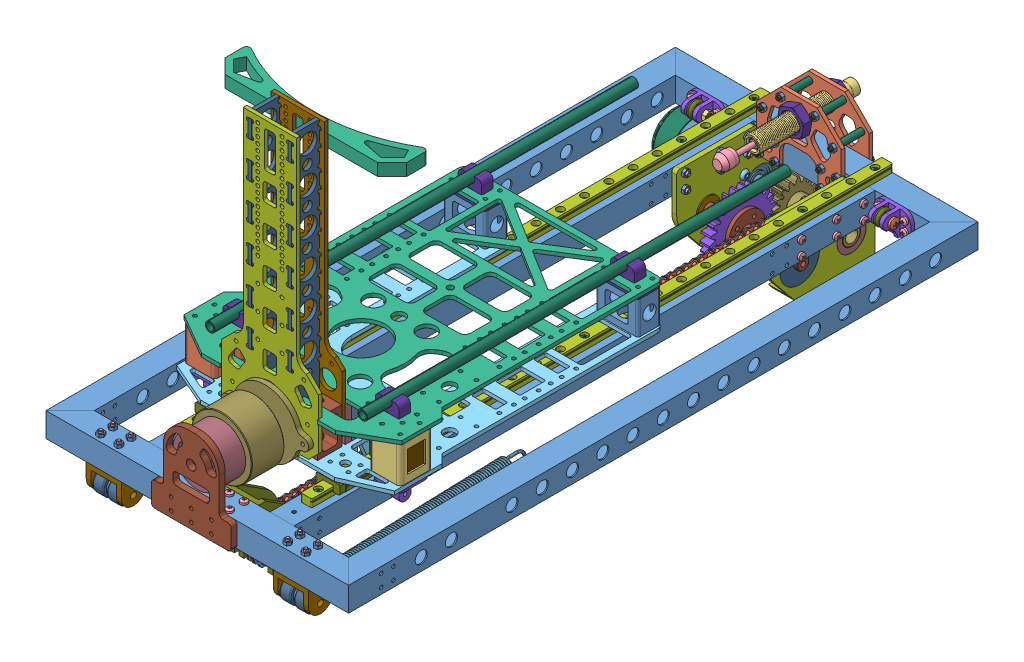
SolidWorks assembly 寒冰射手-wlⅡ-2AT-sc, configuration 默认. Lengths in mm. (continued)
Components (placement in the parent): (continued)
- 内链板T-sc-27: 内链板T-sc [默认] at (-33.1592 30.038 131.3321) x (0 0.000728 1) z (1 0 0) size (12.35 6 4.78)
- 内链板T-sc-28: 内链板T-sc [默认] at (-33.1592 30.0473 144.032) x (0 0.000728 1) z (1 0 0) size (12.35 6 4.78)
- 内链板T-sc-29: 内链板T-sc [默认] at (-33.1592 30.0565 156.732) x (0 0.000728 1) z (1 0 0) size (12.35 6 4.78)
- 内链板T-sc-30: 内链板T-sc [默认] at (-33.1592 30.0658 169.432) x (0 0.000728 1) z (1 0 0) size (12.35 6 4.78)
- 内链板T-sc-31: 内链板T-sc [默认] at (-33.1592 30.075 182.132) x (0 0.000728 1) z (1 0 0) size (12.35 6 4.78)
- 内链板T-sc-32: 内链板T-sc [默认] at (-33.1592 30.0843 194.832) x (0 0.000728 1) z (1 0 0) size (12.35 6 4.78)
- 内链板T-sc-33: 内链板T-sc [默认] at (-33.1592 30.0935 207.532) x (0 0.000728 1) z (1 0 0) size (12.35 6 4.78)
- 内链板T-sc-34: 内链板T-sc [默认] at (-33.1592 29.3036 220.1821) x (0 -0.470065 0.882632) z (1 0 0) size (12.35 6 4.78)
- 内链板T-sc-35: 内链板T-sc [默认] at (-33.1592 21.5108 229.9349) x (0 -0.941992 0.335634) z (1 0 0) size (12.35 6 4.78)
- 内链板T-sc-36: 内链板T-sc [默认] at (-33.1592 9.1815 231.8928) x (0 -0.922274 -0.386537) z (1 0 0) size (12.35 6 4.78)
- 内链板T-sc-37: 内链板T-sc [默认] at (-33.1592 -1.2493 225.0341) x (0 -0.421201 -0.906967) z (1 0 0) size (12.35 6 4.78)
- 内链板T-sc-38: 内链板T-sc [默认] at (-33.1592 -4.4596 212.9475) x (0 0.000726 -1) z (1 0 0) size (12.35 6 4.78)
- 内链板T-sc-39: 内链板T-sc [默认] at (-33.1592 -4.4503 200.2475) x (0 0.000726 -1) z (1 0 0) size (12.35 6 4.78)
- 内链板T-sc-40: 内链板T-sc [默认] at (-33.1592 -4.4411 187.5475) x (0 0.000726 -1) z (1 0 0) size (12.35 6 4.78)
- 内链板T-sc-41: 内链板T-sc [默认] at (-33.1592 -4.4319 174.8475) x (0 0.000726 -1) z (1 0 0) size (12.35 6 4.78)
- 内链板T-sc-42: 内链板T-sc [默认] at (-33.1592 -4.4227 162.1475) x (0 0.000726 -1) z (1 0 0) size (12.35 6 4.78)
- 内链板T-sc-43: 内链板T-sc [默认] at (-33.1592 -4.4135 149.4475) x (0 0.000726 -1) z (1 0 0) size (12.35 6 4.78)
- 内链板T-sc-44: 内链板T-sc [默认] at (-33.1592 -4.4042 136.7475) x (0 0.000726 -1) z (1 0 0) size (12.35 6 4.78)
- 内链板T-sc-45: 内链板T-sc [默认] at (-33.1592 -4.395 124.0475) x (0 0.000726 -1) z (1 0 0) size (12.35 6 4.78)
- 内链板T-sc-46: 内链板T-sc [默认] at (-33.1592 -4.3858 111.3475) x (0 0.000726 -1) z (1 0 0) size (12.35 6 4.78)
- 内链板T-sc-47: 内链板T-sc [默认] at (-33.1592 -4.3766 98.6476) x (0 0.000726 -1) z (1 0 0) size (12.35 6 4.78)
- 内链板T-sc-48: 内链板T-sc [默认] at (-33.1592 -4.3674 85.9476) x (0 0.000726 -1) z (1 0 0) size (12.35 6 4.78)
- 内链板T-sc-49: 内链板T-sc [默认] at (-33.1592 -4.3581 73.2476) x (0 0.000726 -1) z (1 0 0) size (12.35 6 4.78)
- 内链板T-sc-50: 内链板T-sc [默认] at (-33.1592 -4.3489 60.5476) x (0 0.000726 -1) z (1 0 0) size (12.35 6 4.78)
- 内链板T-sc-51: 内链板T-sc [默认] at (-33.1592 -4.3397 47.8476) x (0 0.000726 -1) z (1 0 0) size (12.35 6 4.78)
- 内链板T-sc-52: 内链板T-sc [默认] at (-33.1592 -4.3305 35.1476) x (0 0.000726 -1) z (1 0 0) size (12.35 6 4.78)
- 内链板T-sc-53: 内链板T-sc [默认] at (-33.1592 -4.3212 22.4476) x (0 0.000726 -1) z (1 0 0) size (12.35 6 4.78)
- 内链板T-sc-54: 内链板T-sc [默认] at (-33.1592 -4.312 9.7476) x (0 0.000726 -1) z (1 0 0) size (12.35 6 4.78)
- 内链板T-sc-55: 内链板T-sc [默认] at (-33.1592 -4.3028 -2.9524) x (0 0.000726 -1) z (1 0 0) size (12.35 6 4.78)
- 内链板T-sc-56: 内链板T-sc [默认] at (-33.1592 -4.2936 -15.6524) x (0 0.000726 -1) z (1 0 0) size (12.35 6 4.78)
- 内链板T-sc-57: 内链板T-sc [默认] at (-33.1592 -4.2844 -28.3523) x (0 0.000726 -1) z (1 0 0) size (12.35 6 4.78)
- 内链板T-sc-58: 内链板T-sc [默认] at (-33.1592 -4.2751 -41.0523) x (0 0.000726 -1) z (1 0 0) size (12.35 6 4.78)
- 内链板T-sc-59: 内链板T-sc [默认] at (-33.1592 -4.2659 -53.7523) x (0 0.000726 -1) z (1 0 0) size (12.35 6 4.78)
- 内链板T-sc-60: 内链板T-sc [默认] at (-33.1592 -4.2567 -66.4523) x (0 0.000726 -1) z (1 0 0) size (12.35 6 4.78)
- 内链板T-sc-61: 内链板T-sc [默认] at (-33.1592 -4.2475 -79.1523) x (0 0.000726 -1) z (1 0 0) size (12.35 6 4.78)
- 内链板T-sc-62: 内链板T-sc [默认] at (-33.1592 -4.2383 -91.8523) x (0 0.000726 -1) z (1 0 0) size (12.35 6 4.78)
- 内链板T-sc-63: 内链板T-sc [默认] at (-33.1592 -4.229 -104.5523) x (0 0.000726 -1) z (1 0 0) size (12.35 6 4.78)
- 内链板T-sc-64: 内链板T-sc [默认] at (-33.1592 -4.2198 -117.2523) x (0 0.000726 -1) z (1 0 0) size (12.35 6 4.78)
- 内链板T-sc-65: 内链板T-sc [默认] at (-33.1592 -4.2106 -129.9523) x (0 0.000726 -1) z (1 0 0) size (12.35 6 4.78)
- 内链板T-sc-66: 内链板T-sc [默认] at (-33.1592 -4.2014 -142.6522) x (0 0.000726 -1) z (1 0 0) size (12.35 6 4.78)
- 内链板T-sc-67: 内链板T-sc [默认] at (-33.1592 -4.1922 -155.3522) x (0 0.000726 -1) z (1 0 0) size (12.35 6 4.78)
- 内链板T-sc-68: 内链板T-sc [默认] at (-33.1592 -4.1829 -168.0522) x (0 0.000726 -1) z (1 0 0) size (12.35 6 4.78)
- 内链板T-sc-69: 内链板T-sc [默认] at (-33.1592 -4.1737 -180.7522) x (0 0.000726 -1) z (1 0 0) size (12.35 6 4.78)
- 内链板T-sc-70: 内链板T-sc [默认] at (-33.1592 -4.1645 -193.4522) x (0 0.02154 -0.999768) z (1 0 0) size (12.35 6 4.78)
- 内链板T-sc-71: 内链板T-sc [默认] at (-33.1592 -2.0684 -205.8409) x (0 0.636425 -0.771338) z (1 0 0) size (12.35 6 4.78)
- 内链板T-sc-72: 内链板T-sc [默认] at (-33.1592 7.531 -213.8097) x (0 0.991746 -0.12822) z (1 0 0) size (12.35 6 4.78)
- 内链板T-sc-73: 内链板T-sc [默认] at (-33.1592 19.9849 -213.0676) x (0 0.811669 0.584118) z (1 0 0) size (12.35 6 4.78)
- 链齿平钩T-1: 链齿平钩T [默认] at (-33.1492 30.127 90.8901) x (0 -0.000728 -1) z (-1 0 0) size (27.4 8.17 29)
- 链齿平钩下-1: 链齿平钩下 [默认] at (-33.1492 29.8726 66.771) x (0 0.000728 1) z (-1 0 0) size (27.4 4 29)
- 发射托盘-wlⅡ-1: 发射托盘-wlⅡ [默认] at (-17.4385 -21.9121 -45.4891) size (180 275 367.06)
  - 发射托盘-wlⅡ11-1: 发射托盘-wlⅡ11 [默认] at (25.4712 86.7307 214.002) x (1 0 0) z (0 1 0) size (180 367.06 246)
    - 发射下平台-wlⅡ11-1: 发射下平台-wlⅡ11 [默认] at (129.5435 38.08 -1.5) size (180 244.52 3)
    - 发射上平台-wlⅡ11-1: 发射上平台-wlⅡ11 [默认] at (-66.2821 39.0561 31.5) x (-1 0 0) z (0 0 1) size (180 243.55 3)
    - 后推板-wlⅡ11-1: 后推板-wlⅡ11 [默认] at (-54.3543 -31.5036 108.5) x (-1 0 0) z (0 0 -1) size (80 3 230)
    - 弹射拉线小座子-wlⅡ11-1: 弹射拉线小座子-wlⅡ11 [默认] at (-136.5321 -0.5634 -1.5) x (0 -1 0) z (1 0 0) size (24 18 23)
    - 弹射拉线小座子-wlⅡ11-2: 弹射拉线小座子-wlⅡ11 [默认] at (17.9679 -0.5634 -1.5) x (0 -1 0) z (1 0 0) size (24 18 23)
    - 前推板-wlⅡ11-1: 前推板-wlⅡ11 [默认] at (-19.2821 -8.5036 1.5) x (-1 0 0) z (0 0 -1) size (73 3 218)
    - 侧向加固板-wlⅡ11-1: 侧向加固板-wlⅡ11 [默认] at (-41.2821 -8.5036 31.6) x (0 -1 0) z (0 0 -1) size (26 3 194.4)
    - 侧向加固板-wlⅡ11-2: 侧向加固板-wlⅡ11 [默认] at (-74.2821 -8.5036 31.6) x (0 -1 0) z (0 0 -1) size (26 3 194.4)
    - 推板固定件-wlⅡ11-1: 推板固定件-wlⅡ11 [默认] at (-22.7821 -18.5036 16.5) x (0 -1 0) z (-1 0 0) size (20 30 73)
    - 电磁吸铁80kg配套-wlⅡ11-1: 电磁吸铁80kg配套-wlⅡ11 [默认] at (-59.2821 -35.5036 14) x (1 0 0) z (0 1 0) size (72 54 4)
    - 8mm发泡硅胶-wlⅡ11-1: 8mm发泡硅胶-wlⅡ11 [默认] at (-59.2821 -8.5036 16.5) size (73 8 30)
    - 8mm聚氨酯-wlⅡ11-1: 8mm聚氨酯-wlⅡ11 [默认] at (-59.2821 -0.5036 16.5) size (73 8 30)
    - 碳管300-wlⅡ11-1: 碳管300-wlⅡ11 [默认] at (-121.7821 331.5561 42.5) x (1 0 0) z (0 -1 0) size (8 8 350)
    - 碳管300-wlⅡ11-2: 碳管300-wlⅡ11 [默认] at (4.2179 331.5561 42.5) x (0.546685 0 0.837338) z (0 -1 0) size (8 8 350)
    - 纵向滑块9mm-wlⅡ11-1: 纵向滑块9mm-wlⅡ11 [默认] at (-109.2822 -33.5634 -9.5) x (1 0 0) z (0 -1 0) size (20 8 28.9)
    - 纵向滑块9mm-wlⅡ11-2: 纵向滑块9mm-wlⅡ11 [默认] at (-9.2819 -33.5634 -9.5) x (1 0 0) z (0 -1 0) size (20 8 28.9)
    - 纵向滑块9mm-wlⅡ11-3: 纵向滑块9mm-wlⅡ11 [默认] at (-109.2822 32.5366 -9.5) x (1 0 0) z (0 -1 0) size (20 8 28.9)
    - 纵向滑块9mm-wlⅡ11-4: 纵向滑块9mm-wlⅡ11 [默认] at (-9.2819 32.5366 -9.5) x (1 0 0) z (0 -1 0) size (20 8 28.9)
    - 碳管夹2改1-1: 碳管夹2改1 [默认] at (4.2179 6.5561 28.5) x (0 1 0) z (0 0 1) size (19 35 16)
    - 垫块1-1: 垫块1 [默认] at (17.9679 -0.5634 1.5) x (0 -1 0) z (0 0 1) size (23 22 30)
    - 碳管夹2改1-2: 碳管夹2改1 [默认] at (4.2179 201.0156 28.5) x (0 1 0) z (0 0 1) size (19 35 16)
    - 垫块改1-1: 垫块改1 [默认] at (4.2179 201.0156 1.5) size (35 19 27)
    - 方碳管固定1-1: 方碳管固定1 [默认] at (-130.2821 1.5561 1.5) size (37 30 30)
    - 方碳管固定右1-2: 方碳管固定右1 [默认] at (11.7179 1.5561 31.5) x (-1 0 0) z (0 0 -1) size (37 30 30)
    - 加固碳板1-1: 加固碳板1 [默认] at (-42.2822 22.9964 -4.5) size (35 50 3)
  - 平台直钩1-1: 平台直钩1 [默认] at (-16.811 82.2307 191.0056) x (1 0 0) z (0 -1 0) size (26 20 44)
  - 垫块改1-1: 垫块改1 [默认] at (-96.3109 88.2307 12.9864) x (1 0 0) z (0 1 0) size (35 19 27)
  - 碳管夹2改1-1: 碳管夹2改1 [默认] at (-96.3109 115.2307 12.9864) x (0 0 -1) z (0 1 0) size (19 35 16)
  - 碳管夹2改1-2: 碳管夹2改1 [默认] at (-96.3109 115.2307 207.4459) x (0 0 -1) z (0 1 0) size (19 35 16)
  - 小推爪-280--1: 小推爪-280- [默认] at (-33.8109 293.2307 204.9956) size (150 10 29.67)
Mates (geometry in assembly coordinates):
- 重合1: coincident anti-aligned: plane of 发射架-wlⅡ-2AT-sc-1 through (63.7508 32.8186 -260) normal (0 0 -1); plane of 缓冲器固定板-wlⅡ-2AT-sc-1 through (-86.2492 32.8186 -260) normal (0 0 1)
- 重合2: coincident aligned: plane of 发射架-wlⅡ-2AT-sc-1 through (63.7508 32.8186 -240) normal (0 -1 0); plane of 缓冲器固定板-wlⅡ-2AT-sc-1 through (-86.2492 32.8186 -260) normal (0 -1 0)
- 宽度1: width anti-aligned: plane of 发射架-wlⅡ-2AT-sc-1 through (-91.2492 32.8186 250) normal (1 0 0); plane of 发射架-wlⅡ-2AT-sc-1 through (-11.2492 32.8186 250) normal (-1 0 0); plane of 缓冲器固定板-wlⅡ-2AT-sc-1 through (-86.2492 32.8186 -260) normal (-1 0 0); plane of 缓冲器固定板-wlⅡ-2AT-sc-1 through (-16.2492 32.8186 -260) normal (1 0 0)
- 重合4: coincident anti-aligned: plane of 发射架-wlⅡ-2AT-sc-1 through (63.7508 32.8186 -240) normal (0 0 1); plane of 缓冲器固定板-wlⅡ-2AT-sc-3 through (-86.2492 32.8186 -240) normal (0 0 -1)
- 重合5: coincident aligned: plane of 发射架-wlⅡ-2AT-sc-1 through (63.7508 32.8186 -240) normal (0 -1 0); plane of 缓冲器固定板-wlⅡ-2AT-sc-3 through (-86.2492 32.8186 -237) normal (0 -1 0)
- 重合6: coincident aligned: plane of 缓冲器固定板-wlⅡ-2AT-sc-1 through (-16.2492 32.8186 -260) normal (1 0 0); plane of 缓冲器固定板-wlⅡ-2AT-sc-3 through (-16.2492 32.8186 -237) normal (1 0 0)
- 同心1: concentric aligned: cylinder of 缓冲器固定板-wlⅡ-2AT-sc-3 through (-51.2492 76.3186 -237) axis (0 0 -1) radius 7; cylinder of 阻尼器-wlⅡ-2AT-sc-1/阻尼器缸体-wlⅡ-2AT-sc-1 through (-51.2492 76.3186 -270) axis (0 0 -1) radius 5.875
- 同心2: concentric aligned: cylinder of 缓冲器固定板-wlⅡ-2AT-sc-1 through (-51.2492 76.3186 -260) axis (0 0 -1) radius 7; cylinder of GB／T6172．1-2000六角薄螺母A级和B级(M14)-wlⅡ-2AT-sc-1 through (-51.2492 76.3186 -263) axis (0 0 -1) radius 7
- 重合7: coincident anti-aligned: plane of 缓冲器固定板-wlⅡ-2AT-sc-1 through (-86.2492 32.8186 -263) normal (0 0 -1); plane of GB／T6172．1-2000六角薄螺母A级和B级(M14)-wlⅡ-2AT-sc-1 through (-49.1953 87.8115 -263) normal (0 0 1)
- 重合9: coincident aligned: circle of 阻尼器-wlⅡ-2AT-sc-1/阻尼器缸体-wlⅡ-2AT-sc-1; plane of GB／T6172．1-2000六角薄螺母A级和B级(M14)-wlⅡ-2AT-sc-1 through (-49.1953 87.8115 -270) normal (0 0 -1)
- 同心4: concentric aligned: cylinder of 阻尼器-wlⅡ-2AT-sc-1/阻尼器缸体-wlⅡ-2AT-sc-1 through (-51.2492 76.3186 -276.1) axis (0 0 -1) radius 5.875; cylinder of GB／T6172．1-2000六角薄螺母A级和B级(M14)-wlⅡ-2AT-sc-2 through (-51.2492 76.3186 -230) axis (0 0 -1) radius 7
- 重合10: coincident anti-aligned: plane of 缓冲器固定板-wlⅡ-2AT-sc-3 through (-86.2492 32.8186 -237) normal (0 0 1); plane of GB／T6172．1-2000六角薄螺母A级和B级(M14)-wlⅡ-2AT-sc-2 through (-49.1953 87.8115 -237) normal (0 0 -1)
- 重合11: coincident anti-aligned: plane of 发射架-wlⅡ-2AT-sc-1 through (-11.2492 52.8186 250) normal (0 1 0); plane of 发射导轨-wlⅡ-2AT-sc-1 through (-5.7492 52.8186 220) normal (0 -1 0)
- 重合14: coincident anti-aligned: plane of 发射架-wlⅡ-2AT-sc-1 through (-111.2492 52.8186 250) normal (0 1 0); plane of 发射导轨-wlⅡ-2AT-sc-2 through (-105.7492 52.8186 220) normal (0 -1 0)
- 宽度2: width anti-aligned: plane of 发射导轨-wlⅡ-2AT-sc-2 through (-105.7492 52.8186 220) normal (-1 0 0); plane of 发射导轨-wlⅡ-2AT-sc-2 through (-96.7492 52.8186 220) normal (1 0 0); plane of 发射架-wlⅡ-2AT-sc-1 through (-91.2492 32.8186 250) normal (1 0 0); plane of 发射架-wlⅡ-2AT-sc-1 through (-111.2492 32.8186 250) normal (-1 0 0)
- 宽度3: width anti-aligned: plane of 发射架-wlⅡ-2AT-sc-1 through (-11.2492 32.8186 250) normal (-1 0 0); plane of 发射架-wlⅡ-2AT-sc-1 through (8.7508 32.8186 250) normal (1 0 0); plane of 发射导轨-wlⅡ-2AT-sc-1 through (3.2508 52.8186 220) normal (1 0 0); plane of 发射导轨-wlⅡ-2AT-sc-1 through (-5.7492 52.8186 220) normal (-1 0 0)
- 重合15: coincident anti-aligned: plane of 缓冲器固定板-wlⅡ-2AT-sc-1 through (-86.2492 32.8186 -260) normal (0 0 1); plane of 20尼龙柱-wlⅡ-2AT-sc-1 through (-65.1781 84.8186 -260) normal (0 0 -1)
- 同心5: concentric anti-aligned: cylinder of 缓冲器固定板-wlⅡ-2AT-sc-1 through (-65.1781 84.8186 -260) axis (0 0 -1) radius 1.5; cylinder of 20尼龙柱-wlⅡ-2AT-sc-1 through (-65.1781 84.8186 -260) axis (0 0 1) radius 1.5
- 同心6: concentric anti-aligned: cylinder of 缓冲器固定板-wlⅡ-2AT-sc-1 through (-80.2492 69.7475 -260) axis (0 0 -1) radius 1.5; cylinder of 20尼龙柱-wlⅡ-2AT-sc-3 through (-80.2492 69.7475 -260) axis (0 0 1) radius 1.5
- 重合16: coincident anti-aligned: plane of 缓冲器固定板-wlⅡ-2AT-sc-1 through (-86.2492 32.8186 -260) normal (0 0 1); plane of 20尼龙柱-wlⅡ-2AT-sc-3 through (-80.2492 69.7475 -260) normal (0 0 -1)
- 同心7: concentric anti-aligned: cylinder of 缓冲器固定板-wlⅡ-2AT-sc-3 through (-37.3203 84.8186 -237) axis (0 0 -1) radius 1.5; cylinder of 20尼龙柱-wlⅡ-2AT-sc-4 through (-37.3203 84.8186 -260) axis (0 0 1) radius 1.5
- 重合17: coincident anti-aligned: plane of 缓冲器固定板-wlⅡ-2AT-sc-1 through (-86.2492 32.8186 -260) normal (0 0 1); plane of 20尼龙柱-wlⅡ-2AT-sc-4 through (-37.3203 84.8186 -260) normal (0 0 -1)
- 同心8: concentric anti-aligned: cylinder of 缓冲器固定板-wlⅡ-2AT-sc-1 through (-22.2492 69.7475 -260) axis (0 0 -1) radius 1.5; cylinder of 20尼龙柱-wlⅡ-2AT-sc-2 through (-22.2492 69.7475 -260) axis (0 0 1) radius 1.5
- 重合18: coincident anti-aligned: plane of 缓冲器固定板-wlⅡ-2AT-sc-1 through (-86.2492 32.8186 -260) normal (0 0 1); plane of 20尼龙柱-wlⅡ-2AT-sc-2 through (-22.2492 69.7475 -260) normal (0 0 -1)
- 重合19: coincident anti-aligned: plane of 发射架-wlⅡ-2AT-sc-1 through (63.7508 32.8186 -240) normal (0 0 1); plane of 拉线座子-wlⅡ-2AT-sc-1 through (26.0008 52.8186 -240) normal (0 0 -1)
- 重合20: coincident aligned: plane of 发射架-wlⅡ-2AT-sc-1 through (63.7508 32.8186 -240) normal (0 -1 0); plane of 拉线座子-wlⅡ-2AT-sc-1 through (45.3335 32.8186 -223) normal (0 -1 0)
- 重合21: coincident anti-aligned: plane of 发射架-wlⅡ-2AT-sc-1 through (63.7508 32.8186 -240) normal (0 0 1); plane of 拉线座子-wlⅡ-2AT-sc-2 through (-128.4992 52.8186 -240) normal (0 0 -1)
- 重合22: coincident aligned: plane of 发射架-wlⅡ-2AT-sc-1 through (63.7508 52.8186 -240) normal (0 1 0); plane of 拉线座子-wlⅡ-2AT-sc-2 through (-128.4992 52.8186 -231.5) normal (0 1 0)
- 距离1: distance = 2 mm anti-aligned: plane of 发射架-wlⅡ-2AT-sc-1 through (-111.2492 32.8186 250) normal (-1 0 0); plane of 拉线座子-wlⅡ-2AT-sc-2 through (-113.2492 25.8186 -237) normal (1 0 0)
- 距离2: distance = 2 mm anti-aligned: plane of 发射架-wlⅡ-2AT-sc-1 through (8.7508 32.8186 250) normal (1 0 0); plane of 拉线座子-wlⅡ-2AT-sc-1 through (10.7508 25.8186 -237) normal (-1 0 0)
- 同心9: concentric aligned: cylinder of 拉线座子-wlⅡ-2AT-sc-2 through (-122.2492 46.0686 -231) axis (-1 0 0) radius 2; cylinder of 现有线轮轴承-wlⅡ-2AT-sc-1 through (-194.9309 46.0686 -231) axis (-1 0 0) radius 2
- 同心10: concentric aligned: cylinder of 拉线座子-wlⅡ-2AT-sc-1 through (32.2508 46.0686 -231) axis (-1 0 0) radius 2; cylinder of 现有线轮轴承-wlⅡ-2AT-sc-2 through (-40.4309 46.0686 -231) axis (-1 0 0) radius 2
- 宽度4: width anti-aligned: plane of 拉线座子-wlⅡ-2AT-sc-2 through (-131.7492 52.8186 -231.5) normal (1 0 0); plane of 拉线座子-wlⅡ-2AT-sc-2 through (-125.2492 52.8186 -231.5) normal (-1 0 0); plane of 现有线轮轴承-wlⅡ-2AT-sc-1 through (-131.4992 48.0684 -231.0238) normal (-1 0 0); plane of 现有线轮轴承-wlⅡ-2AT-sc-1 through (-125.4992 48.0684 -231.0238) normal (1 0 0)
- 宽度6: width anti-aligned: plane of 拉线座子-wlⅡ-2AT-sc-1 through (29.2508 52.8186 -231.5) normal (-1 0 0); plane of 拉线座子-wlⅡ-2AT-sc-1 through (22.7508 52.8186 -231.5) normal (1 0 0); plane of 现有线轮轴承-wlⅡ-2AT-sc-2 through (29.0008 48.0574 -230.7888) normal (1 0 0); plane of 现有线轮轴承-wlⅡ-2AT-sc-2 through (23.0008 48.0574 -230.7888) normal (-1 0 0)
- 宽度7: width anti-aligned: plane of 拉簧座子-wlⅡ-2AT-sc-1 through (36.5008 10.8186 260) normal (-1 0 0); plane of 拉簧座子-wlⅡ-2AT-sc-1 through (15.5008 10.8186 240) normal (1 0 0); plane of 拉线座子-wlⅡ-2AT-sc-1 through (19.7508 52.8186 -231.5) normal (-1 0 0); plane of 拉线座子-wlⅡ-2AT-sc-1 through (32.2508 52.8186 -231.5) normal (1 0 0)
- 宽度8: width anti-aligned: plane of 拉簧座子-wlⅡ-2AT-sc-2 through (-117.9992 10.8186 260) normal (-1 0 0); plane of 拉簧座子-wlⅡ-2AT-sc-2 through (-138.9992 10.8186 240) normal (1 0 0); plane of 拉线座子-wlⅡ-2AT-sc-2 through (-134.7492 52.8186 -231.5) normal (-1 0 0); plane of 拉线座子-wlⅡ-2AT-sc-2 through (-122.2492 52.8186 -231.5) normal (1 0 0)
- 重合27: coincident anti-aligned: plane of 拉簧座子-wlⅡ-2AT-sc-2 through (-138.9992 10.8186 240) normal (1 0 0); plane of 弹簧限位件-wlⅡ-2AT-sc-1 through (-138.9992 18.3186 250) normal (-1 0 0)
- 同心11: concentric anti-aligned: cylinder of 拉簧座子-wlⅡ-2AT-sc-2 through (-113.9992 18.3186 250) axis (-1 0 0) radius 2.5; cylinder of 弹簧限位件-wlⅡ-2AT-sc-1 through (-138.9992 18.3186 250) axis (1 0 0) radius 4.15
- 同心12: concentric anti-aligned: cylinder of 拉簧座子-wlⅡ-2AT-sc-2 through (-113.9992 18.3186 250) axis (-1 0 0) radius 2.5; cylinder of 弹簧限位件-wlⅡ-2AT-sc-2 through (-126.9992 18.3186 250) axis (1 0 0) radius 4.15
- 重合28: coincident anti-aligned: plane of 拉簧座子-wlⅡ-2AT-sc-2 through (-117.9992 10.8186 260) normal (-1 0 0); plane of 弹簧限位件-wlⅡ-2AT-sc-2 through (-117.9992 18.3186 250) normal (1 0 0)
- 同心13: concentric anti-aligned: cylinder of 拉簧座子-wlⅡ-2AT-sc-1 through (40.5008 18.3186 250) axis (-1 0 0) radius 2.5; cylinder of 弹簧限位件-wlⅡ-2AT-sc-3 through (27.5008 18.3186 250) axis (1 0 0) radius 4.15
- 重合29: coincident anti-aligned: plane of 拉簧座子-wlⅡ-2AT-sc-1 through (36.5008 10.8186 260) normal (-1 0 0); plane of 弹簧限位件-wlⅡ-2AT-sc-3 through (36.5008 18.3186 250) normal (1 0 0)
- 重合30: coincident anti-aligned: plane of 拉簧座子-wlⅡ-2AT-sc-1 through (15.5008 10.8186 240) normal (1 0 0); plane of 弹簧限位件-wlⅡ-2AT-sc-4 through (15.5008 18.3186 250) normal (-1 0 0)
- 同心14: concentric anti-aligned: cylinder of 拉簧座子-wlⅡ-2AT-sc-1 through (40.5008 18.3186 250) axis (-1 0 0) radius 2.5; cylinder of 弹簧限位件-wlⅡ-2AT-sc-4 through (15.5008 18.3186 250) axis (1 0 0) radius 4.15
- 重合31: coincident aligned: plane of 发射架-wlⅡ-2AT-sc-1 through (63.7508 32.8186 -260) normal (0 0 -1); plane of 发射导轨-wlⅡ-2AT-sc-2 through (-101.2492 56.482 -260) normal (0 0 -1)
- 重合32: coincident aligned: plane of 发射架-wlⅡ-2AT-sc-1 through (63.7508 32.8186 -260) normal (0 0 -1); plane of 发射导轨-wlⅡ-2AT-sc-1 through (-1.2492 56.482 -260) normal (0 0 -1)
- 重合33: coincident anti-aligned: plane of 电磁吸盘固定板-wlⅡ-2AT-sc-1 through (-51.2492 67.8186 260) normal (0 0 -1); plane of 发射架-wlⅡ-2AT-sc-1 through (-166.2492 32.8186 260) normal (0 0 1)
- 宽度9: width aligned: plane of 发射架-wlⅡ-2AT-sc-1 through (-11.2492 32.8186 250) normal (-1 0 0); plane of 发射架-wlⅡ-2AT-sc-1 through (-91.2492 32.8186 250) normal (1 0 0); plane of 电磁吸盘固定板-wlⅡ-2AT-sc-1 through (-74.2492 102.8186 260) normal (-1 0 0); plane of 电磁吸盘固定板-wlⅡ-2AT-sc-1 through (-28.2492 102.8186 260) normal (1 0 0)
- 同心15: concentric aligned: cylinder of 电磁吸盘固定板-wlⅡ-2AT-sc-1 through (-51.2492 78.8186 260) axis (0 0 1) radius 4; cylinder of 电磁铁开关80kg-wlⅡ-2AT-sc-1 through (-51.2492 78.8186 228) axis (0 0 1) radius 4
- 重合40: coincident aligned: plane of 发射架-wlⅡ-2AT-sc-1 through (-166.2492 32.8186 240) normal (0 -1 0); plane of 电磁吸盘固定板-wlⅡ-2AT-sc-1 through (-74.2492 32.8186 260) normal (0 -1 0)
- 重合41: coincident anti-aligned: plane of 发射架-wlⅡ-2AT-sc-1 through (-166.2492 32.8186 240) normal (0 -1 0); plane of 拉簧座子-wlⅡ-2AT-sc-1 through (26.0008 32.8186 250) normal (0 1 0)
- 重合42: coincident aligned: plane of 发射架-wlⅡ-2AT-sc-1 through (-166.2492 32.8186 260) normal (0 0 1); plane of 拉簧座子-wlⅡ-2AT-sc-1 through (26.0008 28.8186 260) normal (0 0 1)
- 重合43: coincident anti-aligned: plane of 发射架-wlⅡ-2AT-sc-1 through (-166.2492 32.8186 240) normal (0 -1 0); plane of 拉簧座子-wlⅡ-2AT-sc-2 through (-128.4992 32.8186 250) normal (0 1 0)
- 重合44: coincident aligned: plane of 发射架-wlⅡ-2AT-sc-1 through (-166.2492 32.8186 260) normal (0 0 1); plane of 拉簧座子-wlⅡ-2AT-sc-2 through (-128.4992 28.8186 260) normal (0 0 1)
- 同心17: concentric anti-aligned: cylinder of 电磁吸盘固定板-wlⅡ-2AT-sc-1 through (-51.2492 78.8186 260) axis (0 0 1) radius 4; cylinder of 行程调节块-wlⅡ-2AT-sc-1 through (-51.2492 78.8186 260) axis (0 0 -1) radius 4
- 重合49: coincident anti-aligned: plane of 电磁吸盘固定板-wlⅡ-2AT-sc-1 through (-51.2492 67.8186 260) normal (0 0 -1); plane of 行程调节块-wlⅡ-2AT-sc-1 through (-51.2492 78.8186 260) normal (0 0 1)
- 重合50: coincident anti-aligned: plane of 电磁铁开关80kg-wlⅡ-2AT-sc-1 through (-51.2492 78.8186 240) normal (0 0 1); plane of 行程调节块-wlⅡ-2AT-sc-1 through (-51.2492 78.8186 240) normal (0 0 -1)
- 同心26: concentric aligned: cylinder of 缓冲器固定板-wlⅡ-2AT-sc-1 through (-65.1781 84.8186 -260) axis (0 0 -1) radius 1.5; cylinder of GB／T818-2000十字槽盘头螺钉M3×30-wlⅡ-2AT-sc-1 through (-65.1781 84.8186 -266.7318) axis (0 0 -1) radius 1.5
- 重合71: coincident anti-aligned: plane of 缓冲器固定板-wlⅡ-2AT-sc-1 through (-86.2492 32.8186 -263) normal (0 0 -1); plane of GB／T818-2000十字槽盘头螺钉M3×30-wlⅡ-2AT-sc-1 through (-66.6512 85.853 -263) normal (0 0 1)
- 同心27: concentric aligned: cylinder of 缓冲器固定板-wlⅡ-2AT-sc-1 through (-80.2492 69.7475 -260) axis (0 0 -1) radius 1.5; cylinder of GB／T818-2000十字槽盘头螺钉M3×30-wlⅡ-2AT-sc-2 through (-80.2492 69.7475 -266.7318) axis (0 0 -1) radius 1.5
- 同心28: concentric aligned: cylinder of 缓冲器固定板-wlⅡ-2AT-sc-1 through (-37.3203 84.8186 -260) axis (0 0 -1) radius 1.5; cylinder of GB／T818-2000十字槽盘头螺钉M3×30-wlⅡ-2AT-sc-3 through (-37.3203 84.8186 -266.7318) axis (0 0 -1) radius 1.5
- 同心29: concentric aligned: cylinder of 缓冲器固定板-wlⅡ-2AT-sc-1 through (-22.2492 69.7475 -260) axis (0 0 -1) radius 1.5; cylinder of GB／T818-2000十字槽盘头螺钉M3×30-wlⅡ-2AT-sc-4 through (-22.2492 69.7475 -266.7318) axis (0 0 -1) radius 1.5
- 同心30: concentric anti-aligned: cylinder of 缓冲器固定板-wlⅡ-2AT-sc-1 through (-83.2492 49.8186 -263) axis (0 0 1) radius 1.5; cylinder of GB／T818-2000十字槽盘头螺钉M3×30-wlⅡ-2AT-sc-12 through (-83.2492 49.8186 -266.7318) axis (0 0 -1) radius 1.5
- 同心31: concentric anti-aligned: cylinder of 缓冲器固定板-wlⅡ-2AT-sc-1 through (-83.2492 35.8186 -263) axis (0 0 1) radius 1.5; cylinder of GB／T818-2000十字槽盘头螺钉M3×30-wlⅡ-2AT-sc-11 through (-83.2492 35.8186 -266.7318) axis (0 0 -1) radius 1.5
- 同心32: concentric anti-aligned: cylinder of 缓冲器固定板-wlⅡ-2AT-sc-1 through (-70.2492 35.8186 -263) axis (0 0 1) radius 1.5; cylinder of GB／T818-2000十字槽盘头螺钉M3×30-wlⅡ-2AT-sc-8 through (-70.2492 35.8186 -266.7318) axis (0 0 -1) radius 1.5
- 同心33: concentric anti-aligned: cylinder of 缓冲器固定板-wlⅡ-2AT-sc-1 through (-70.2492 49.8186 -263) axis (0 0 1) radius 1.5; cylinder of GB／T818-2000十字槽盘头螺钉M3×30-wlⅡ-2AT-sc-9 through (-70.2492 49.8186 -266.7318) axis (0 0 -1) radius 1.5
- 同心34: concentric anti-aligned: cylinder of 缓冲器固定板-wlⅡ-2AT-sc-1 through (-32.2492 35.8186 -263) axis (0 0 1) radius 1.5; cylinder of GB／T818-2000十字槽盘头螺钉M3×30-wlⅡ-2AT-sc-7 through (-32.2492 35.8186 -266.7318) axis (0 0 -1) radius 1.5
- 同心35: concentric anti-aligned: cylinder of 缓冲器固定板-wlⅡ-2AT-sc-1 through (-19.2492 35.8186 -263) axis (0 0 1) radius 1.5; cylinder of GB／T818-2000十字槽盘头螺钉M3×30-wlⅡ-2AT-sc-6 through (-19.2492 35.8186 -266.7318) axis (0 0 -1) radius 1.5
- 同心36: concentric anti-aligned: cylinder of 缓冲器固定板-wlⅡ-2AT-sc-1 through (-19.2492 49.8186 -263) axis (0 0 1) radius 1.5; cylinder of GB／T818-2000十字槽盘头螺钉M3×30-wlⅡ-2AT-sc-13 through (-19.2492 49.8186 -266.7318) axis (0 0 -1) radius 1.5
- 同心37: concentric anti-aligned: cylinder of 缓冲器固定板-wlⅡ-2AT-sc-1 through (-32.2492 49.8186 -263) axis (0 0 1) radius 1.5; cylinder of GB／T818-2000十字槽盘头螺钉M3×30-wlⅡ-2AT-sc-10 through (-32.2492 49.8186 -266.7318) axis (0 0 -1) radius 1.5
- 重合72: coincident anti-aligned: plane of 缓冲器固定板-wlⅡ-2AT-sc-1 through (-86.2492 32.8186 -263) normal (0 0 -1); plane of GB／T818-2000十字槽盘头螺钉M3×30-wlⅡ-2AT-sc-2 through (-81.7223 70.7819 -263) normal (0 0 1)
- 重合73: coincident anti-aligned: plane of 缓冲器固定板-wlⅡ-2AT-sc-1 through (-86.2492 32.8186 -263) normal (0 0 -1); plane of GB／T818-2000十字槽盘头螺钉M3×30-wlⅡ-2AT-sc-9 through (-72.0172 50.1566 -263) normal (0 0 1)
- 重合74: coincident anti-aligned: plane of 缓冲器固定板-wlⅡ-2AT-sc-1 through (-86.2492 32.8186 -263) normal (0 0 -1); plane of GB／T818-2000十字槽盘头螺钉M3×30-wlⅡ-2AT-sc-12 through (-84.7223 50.853 -263) normal (0 0 1)
- 重合75: coincident anti-aligned: plane of 缓冲器固定板-wlⅡ-2AT-sc-1 through (-86.2492 32.8186 -263) normal (0 0 -1); plane of GB／T818-2000十字槽盘头螺钉M3×30-wlⅡ-2AT-sc-11 through (-84.7223 36.853 -263) normal (0 0 1)
- 重合76: coincident anti-aligned: plane of 缓冲器固定板-wlⅡ-2AT-sc-1 through (-86.2492 32.8186 -263) normal (0 0 -1); plane of GB／T818-2000十字槽盘头螺钉M3×30-wlⅡ-2AT-sc-8 through (-71.7223 36.853 -263) normal (0 0 1)
- 重合77: coincident anti-aligned: plane of 缓冲器固定板-wlⅡ-2AT-sc-1 through (-86.2492 32.8186 -263) normal (0 0 -1); plane of GB／T818-2000十字槽盘头螺钉M3×30-wlⅡ-2AT-sc-10 through (-33.7223 50.853 -263) normal (0 0 1)
- 重合78: coincident aligned: plane of 缓冲器固定板-wlⅡ-2AT-sc-1 through (-86.2492 32.8186 -263) normal (0 0 -1); circle of GB／T818-2000十字槽盘头螺钉M3×30-wlⅡ-2AT-sc-7
- 重合79: coincident anti-aligned: plane of 缓冲器固定板-wlⅡ-2AT-sc-1 through (-86.2492 32.8186 -263) normal (0 0 -1); plane of GB／T818-2000十字槽盘头螺钉M3×30-wlⅡ-2AT-sc-13 through (-20.7223 50.853 -263) normal (0 0 1)
- 重合80: coincident anti-aligned: plane of 缓冲器固定板-wlⅡ-2AT-sc-1 through (-86.2492 32.8186 -263) normal (0 0 -1); plane of GB／T818-2000十字槽盘头螺钉M3×30-wlⅡ-2AT-sc-6 through (-20.7223 36.853 -263) normal (0 0 1)
- 重合81: coincident anti-aligned: plane of 缓冲器固定板-wlⅡ-2AT-sc-1 through (-86.2492 32.8186 -263) normal (0 0 -1); plane of GB／T818-2000十字槽盘头螺钉M3×30-wlⅡ-2AT-sc-4 through (-23.7223 70.7819 -263) normal (0 0 1)
- 重合82: coincident anti-aligned: plane of 缓冲器固定板-wlⅡ-2AT-sc-1 through (-86.2492 32.8186 -263) normal (0 0 -1); plane of GB／T818-2000十字槽盘头螺钉M3×30-wlⅡ-2AT-sc-3 through (-39.1014 85.0787 -263) normal (0 0 1)
- 同心38: concentric aligned: cylinder of GB／T818-2000十字槽盘头螺钉M3×30-wlⅡ-2AT-sc-6 through (-19.2492 35.8186 -266.7318) axis (0 0 -1) radius 1.5; cylinder of GB／T6170-20001型六角螺母A级和B级M3-wlⅡ-2AT-sc-1 through (-19.2492 35.8186 -234.6) axis (0 0 -1) radius 1.5
- 重合83: coincident anti-aligned: plane of 缓冲器固定板-wlⅡ-2AT-sc-3 through (-86.2492 32.8186 -237) normal (0 0 1); plane of GB／T6170-20001型六角螺母A级和B级M3-wlⅡ-2AT-sc-1 through (-16.6409 37.3108 -237) normal (0 0 -1)
- 同心39: concentric aligned: cylinder of GB／T818-2000十字槽盘头螺钉M3×30-wlⅡ-2AT-sc-7 through (-32.2492 35.8186 -266.7318) axis (0 0 -1) radius 1.5; cylinder of GB／T6170-20001型六角螺母A级和B级M3-wlⅡ-2AT-sc-2 through (-32.2492 35.8186 -234.6) axis (0 0 -1) radius 1.5
- 重合84: coincident anti-aligned: plane of 缓冲器固定板-wlⅡ-2AT-sc-3 through (-86.2492 32.8186 -237) normal (0 0 1); plane of GB／T6170-20001型六角螺母A级和B级M3-wlⅡ-2AT-sc-2 through (-29.6409 37.3108 -237) normal (0 0 -1)
- 同心40: concentric aligned: cylinder of GB／T818-2000十字槽盘头螺钉M3×30-wlⅡ-2AT-sc-8 through (-70.2492 35.8186 -266.7318) axis (0 0 -1) radius 1.5; cylinder of GB／T6170-20001型六角螺母A级和B级M3-wlⅡ-2AT-sc-4 through (-70.2492 35.8186 -234.6) axis (0 0 -1) radius 1.5
- 重合85: coincident anti-aligned: plane of 缓冲器固定板-wlⅡ-2AT-sc-3 through (-86.2492 32.8186 -237) normal (0 0 1); plane of GB／T6170-20001型六角螺母A级和B级M3-wlⅡ-2AT-sc-4 through (-67.6409 37.3108 -237) normal (0 0 -1)
- 同心41: concentric aligned: cylinder of GB／T818-2000十字槽盘头螺钉M3×30-wlⅡ-2AT-sc-11 through (-83.2492 35.8186 -266.7318) axis (0 0 -1) radius 1.5; cylinder of GB／T6170-20001型六角螺母A级和B级M3-wlⅡ-2AT-sc-5 through (-83.2492 35.8186 -234.6) axis (0 0 -1) radius 1.5
- 重合86: coincident anti-aligned: plane of 缓冲器固定板-wlⅡ-2AT-sc-3 through (-86.2492 32.8186 -237) normal (0 0 1); plane of GB／T6170-20001型六角螺母A级和B级M3-wlⅡ-2AT-sc-5 through (-80.6409 37.3108 -237) normal (0 0 -1)
- 同心60: concentric aligned: cylinder of GB／T818-2000十字槽盘头螺钉M3×30-wlⅡ-2AT-sc-12 through (-83.2492 49.8186 -266.7318) axis (0 0 -1) radius 1.5; cylinder of GB／T6170-20001型六角螺母A级和B级M3-wlⅡ-2AT-sc-6 through (-83.2492 49.8186 -234.6) axis (0 0 -1) radius 1.5
- 重合104: coincident anti-aligned: plane of 缓冲器固定板-wlⅡ-2AT-sc-3 through (-86.2492 32.8186 -237) normal (0 0 1); plane of GB／T6170-20001型六角螺母A级和B级M3-wlⅡ-2AT-sc-6 through (-80.6409 51.3108 -237) normal (0 0 -1)
- 同心61: concentric aligned: cylinder of GB／T818-2000十字槽盘头螺钉M3×30-wlⅡ-2AT-sc-9 through (-70.2492 49.8186 -266.7318) axis (0 0 -1) radius 1.5; cylinder of GB／T6170-20001型六角螺母A级和B级M3-wlⅡ-2AT-sc-7 through (-70.2492 49.8186 -234.6) axis (0 0 -1) radius 1.5
- 重合105: coincident anti-aligned: plane of 缓冲器固定板-wlⅡ-2AT-sc-3 through (-86.2492 32.8186 -237) normal (0 0 1); plane of GB／T6170-20001型六角螺母A级和B级M3-wlⅡ-2AT-sc-7 through (-67.6409 51.3108 -237) normal (0 0 -1)
- 同心62: concentric aligned: cylinder of GB／T818-2000十字槽盘头螺钉M3×30-wlⅡ-2AT-sc-2 through (-80.2492 69.7475 -266.7318) axis (0 0 -1) radius 1.5; cylinder of GB／T6170-20001型六角螺母A级和B级M3-wlⅡ-2AT-sc-8 through (-80.2492 69.7475 -234.6) axis (0 0 -1) radius 1.5
- 重合106: coincident anti-aligned: plane of 缓冲器固定板-wlⅡ-2AT-sc-3 through (-86.2492 32.8186 -237) normal (0 0 1); plane of GB／T6170-20001型六角螺母A级和B级M3-wlⅡ-2AT-sc-8 through (-77.6409 71.2398 -237) normal (0 0 -1)
- 同心63: concentric aligned: cylinder of GB／T818-2000十字槽盘头螺钉M3×30-wlⅡ-2AT-sc-1 through (-65.1781 84.8186 -266.7318) axis (0 0 -1) radius 1.5; cylinder of GB／T6170-20001型六角螺母A级和B级M3-wlⅡ-2AT-sc-9 through (-65.1781 84.8186 -234.6) axis (0 0 -1) radius 1.5
- 重合107: coincident anti-aligned: plane of 缓冲器固定板-wlⅡ-2AT-sc-3 through (-86.2492 32.8186 -237) normal (0 0 1); plane of GB／T6170-20001型六角螺母A级和B级M3-wlⅡ-2AT-sc-9 through (-62.5698 86.3108 -237) normal (0 0 -1)
- 同心64: concentric aligned: cylinder of GB／T818-2000十字槽盘头螺钉M3×30-wlⅡ-2AT-sc-10 through (-32.2492 49.8186 -266.7318) axis (0 0 -1) radius 1.5; cylinder of GB／T6170-20001型六角螺母A级和B级M3-wlⅡ-2AT-sc-11 through (-32.2492 49.8186 -234.6) axis (0 0 -1) radius 1.5
- 重合109: coincident anti-aligned: plane of 缓冲器固定板-wlⅡ-2AT-sc-3 through (-86.2492 32.8186 -237) normal (0 0 1); plane of GB／T6170-20001型六角螺母A级和B级M3-wlⅡ-2AT-sc-11 through (-29.6409 51.3108 -237) normal (0 0 -1)
- 同心65: concentric aligned: cylinder of GB／T818-2000十字槽盘头螺钉M3×30-wlⅡ-2AT-sc-13 through (-19.2492 49.8186 -266.7318) axis (0 0 -1) radius 1.5; cylinder of GB／T6170-20001型六角螺母A级和B级M3-wlⅡ-2AT-sc-12 through (-19.2492 49.8186 -234.6) axis (0 0 -1) radius 1.5
- 重合110: coincident anti-aligned: plane of 缓冲器固定板-wlⅡ-2AT-sc-3 through (-86.2492 32.8186 -237) normal (0 0 1); plane of GB／T6170-20001型六角螺母A级和B级M3-wlⅡ-2AT-sc-12 through (-16.6409 51.3108 -237) normal (0 0 -1)
- 重合111: coincident anti-aligned: plane of 缓冲器固定板-wlⅡ-2AT-sc-3 through (-86.2492 32.8186 -237) normal (0 0 1); plane of GB／T6170-20001型六角螺母A级和B级M3-wlⅡ-2AT-sc-14 through (-19.6409 71.2398 -237) normal (0 0 -1)
- 同心67: concentric aligned: cylinder of GB／T818-2000十字槽盘头螺钉M3×30-wlⅡ-2AT-sc-3 through (-37.3203 84.8186 -266.7318) axis (0 0 -1) radius 1.5; cylinder of GB／T6170-20001型六角螺母A级和B级M3-wlⅡ-2AT-sc-13 through (-37.3203 84.8186 -234.6) axis (0 0 -1) radius 1.5
- 重合112: coincident anti-aligned: plane of 缓冲器固定板-wlⅡ-2AT-sc-3 through (-86.2492 32.8186 -237) normal (0 0 1); plane of GB／T6170-20001型六角螺母A级和B级M3-wlⅡ-2AT-sc-13 through (-34.712 86.3108 -237) normal (0 0 -1)
- 同心68: concentric aligned: cylinder of 拉线座子-wlⅡ-2AT-sc-2 through (-122.2492 46.0686 -231) axis (-1 0 0) radius 2; cylinder of GB／T818-2000十字槽盘头螺钉M4×16-wlⅡ-2AT-sc-1 through (-139.181 46.0686 -231) axis (-1 0 0) radius 2
- 重合113: coincident anti-aligned: plane of 拉线座子-wlⅡ-2AT-sc-2 through (-134.7492 52.8186 -231.5) normal (-1 0 0); plane of GB／T818-2000十字槽盘头螺钉M4×16-wlⅡ-2AT-sc-1 through (-134.7492 47.9946 -229.6535) normal (1 0 0)
- 同心69: concentric anti-aligned: cylinder of 拉线座子-wlⅡ-2AT-sc-1 through (32.2508 46.0686 -231) axis (-1 0 0) radius 2; cylinder of GB／T818-2000十字槽盘头螺钉M4×16-wlⅡ-2AT-sc-2 through (36.6826 46.0686 -231) axis (1 0 0) radius 2
- 重合114: coincident anti-aligned: plane of 拉线座子-wlⅡ-2AT-sc-1 through (32.2508 52.8186 -231.5) normal (1 0 0); plane of GB／T818-2000十字槽盘头螺钉M4×16-wlⅡ-2AT-sc-2 through (32.2508 46.2936 -233.3392) normal (-1 0 0)
- 同心70: concentric anti-aligned: cylinder of GB／T818-2000十字槽盘头螺钉M4×16-wlⅡ-2AT-sc-1 through (-139.181 46.0686 -231) axis (-1 0 0) radius 2; cylinder of GB／T6170-20001型六角螺母A级和B级M4-wlⅡ-2AT-sc-1 through (-122.2492 46.0686 -231) axis (1 0 0) radius 2
- 重合115: coincident anti-aligned: plane of 拉线座子-wlⅡ-2AT-sc-2 through (-122.2492 52.8186 -231.5) normal (1 0 0); plane of GB／T6170-20001型六角螺母A级和B级M4-wlⅡ-2AT-sc-1 through (-122.2492 46.0425 -224.3663) normal (-1 0 0)
- 同心71: concentric aligned: cylinder of GB／T818-2000十字槽盘头螺钉M4×16-wlⅡ-2AT-sc-2 through (36.6826 46.0686 -231) axis (1 0 0) radius 2; cylinder of GB／T6170-20001型六角螺母A级和B级M4-wlⅡ-2AT-sc-2 through (16.5508 46.0686 -231) axis (1 0 0) radius 2
- 重合116: coincident anti-aligned: plane of 拉线座子-wlⅡ-2AT-sc-1 through (19.7508 52.8186 -231.5) normal (-1 0 0); plane of GB／T6170-20001型六角螺母A级和B级M4-wlⅡ-2AT-sc-2 through (19.7508 46.0425 -224.3663) normal (1 0 0)
- 同心72: concentric aligned: cylinder of GB／T818-2000十字槽盘头螺钉M3×30-wlⅡ-2AT-sc-4 through (-22.2492 69.7475 -266.7318) axis (0 0 -1) radius 1.5; cylinder of GB／T6170-20001型六角螺母A级和B级M3-wlⅡ-2AT-sc-14 through (-22.2492 69.7475 -234.6) axis (0 0 -1) radius 1.5
- 同心73: concentric aligned: cylinder of 弹簧限位件-wlⅡ-2AT-sc-2 through (-126.9992 18.3186 250) axis (1 0 0) radius 4.15; circle of 拉射拉簧-wlⅡ-2AT-sc-1
- 宽度14: width: plane of 拉簧座子-wlⅡ-2AT-sc-2 through (-117.9992 10.8186 260) normal (-1 0 0); plane of 拉簧座子-wlⅡ-2AT-sc-2 through (-138.9992 10.8186 240) normal (1 0 0); cylinder of 拉射拉簧-wlⅡ-2AT-sc-1 through (-128.4992 14.1 241.3569) axis (0 0.999461 0.032825) radius 1
- 同心74: concentric anti-aligned: cylinder of 拉簧座子-wlⅡ-2AT-sc-1 through (40.5008 18.3186 250) axis (-1 0 0) radius 2.5; circle of 拉射拉簧-wlⅡ-2AT-sc-2
- 宽度15: width: plane of 拉簧座子-wlⅡ-2AT-sc-1 through (15.5008 10.8186 240) normal (1 0 0); plane of 拉簧座子-wlⅡ-2AT-sc-1 through (36.5008 10.8186 260) normal (-1 0 0); cylinder of 拉射拉簧-wlⅡ-2AT-sc-2 through (26.0008 14.1 241.3569) axis (0 0.999461 0.032825) radius 1
- 同心79: concentric aligned: cylinder of 发射架-wlⅡ-2AT-sc-1 through (-111.2492 48.8186 -230) axis (1 0 0) radius 1.5; cylinder of GB／T818-2000十字槽盘头螺钉M3×28-wlⅡ-2AT-sc-1 through (12.4826 48.8186 -230) axis (1 0 0) radius 1.5
- 重合120: coincident anti-aligned: plane of 发射架-wlⅡ-2AT-sc-1 through (8.7508 32.8186 250) normal (1 0 0); plane of GB／T818-2000十字槽盘头螺钉M3×28-wlⅡ-2AT-sc-1 through (8.7508 49.9535 -231.3971) normal (-1 0 0)
- 同心80: concentric aligned: cylinder of 发射架-wlⅡ-2AT-sc-1 through (-111.2492 36.8186 -230) axis (1 0 0) radius 1.5; cylinder of GB／T818-2000十字槽盘头螺钉M3×28-wlⅡ-2AT-sc-2 through (12.4826 36.8186 -230) axis (1 0 0) radius 1.5
- 重合121: coincident anti-aligned: plane of 发射架-wlⅡ-2AT-sc-1 through (8.7508 32.8186 250) normal (1 0 0); plane of GB／T818-2000十字槽盘头螺钉M3×28-wlⅡ-2AT-sc-2 through (8.7508 37.9535 -231.3971) normal (-1 0 0)
- 同心81: concentric aligned: cylinder of 发射架-wlⅡ-2AT-sc-1 through (-111.2492 36.8186 -207.5) axis (1 0 0) radius 1.5; cylinder of GB／T818-2000十字槽盘头螺钉M3×28-wlⅡ-2AT-sc-3 through (12.4826 36.8186 -207.5) axis (1 0 0) radius 1.5
- 同心82: concentric aligned: cylinder of 发射架-wlⅡ-2AT-sc-1 through (-111.2492 48.8186 -207.5) axis (1 0 0) radius 1.5; cylinder of GB／T818-2000十字槽盘头螺钉M3×28-wlⅡ-2AT-sc-4 through (12.4826 48.8186 -207.5) axis (1 0 0) radius 1.5
- 同心83: concentric aligned: cylinder of 发射架-wlⅡ-2AT-sc-1 through (-111.2492 36.8186 -178.5) axis (1 0 0) radius 1.5; cylinder of GB／T818-2000十字槽盘头螺钉M3×28-wlⅡ-2AT-sc-6 through (12.4826 36.8186 -178.5) axis (1 0 0) radius 1.5
- 同心84: concentric aligned: cylinder of 发射架-wlⅡ-2AT-sc-1 through (-111.2492 48.8186 -178.5) axis (1 0 0) radius 1.5; cylinder of GB／T818-2000十字槽盘头螺钉M3×28-wlⅡ-2AT-sc-5 through (12.4826 48.8186 -178.5) axis (1 0 0) radius 1.5
- 重合122: coincident anti-aligned: plane of 发射架-wlⅡ-2AT-sc-1 through (8.7508 32.8186 250) normal (1 0 0); plane of GB／T818-2000十字槽盘头螺钉M3×28-wlⅡ-2AT-sc-4 through (8.7508 49.9535 -208.8971) normal (-1 0 0)
- 重合123: coincident anti-aligned: plane of 发射架-wlⅡ-2AT-sc-1 through (8.7508 32.8186 250) normal (1 0 0); plane of GB／T818-2000十字槽盘头螺钉M3×28-wlⅡ-2AT-sc-3 through (8.7508 37.9535 -208.8971) normal (-1 0 0)
- 重合124: coincident anti-aligned: plane of 发射架-wlⅡ-2AT-sc-1 through (8.7508 32.8186 250) normal (1 0 0); plane of GB／T818-2000十字槽盘头螺钉M3×28-wlⅡ-2AT-sc-5 through (8.7508 49.9535 -179.8971) normal (-1 0 0)
- 重合125: coincident anti-aligned: plane of 发射架-wlⅡ-2AT-sc-1 through (8.7508 32.8186 250) normal (1 0 0); plane of GB／T818-2000十字槽盘头螺钉M3×28-wlⅡ-2AT-sc-6 through (8.7508 37.9535 -179.8971) normal (-1 0 0)
